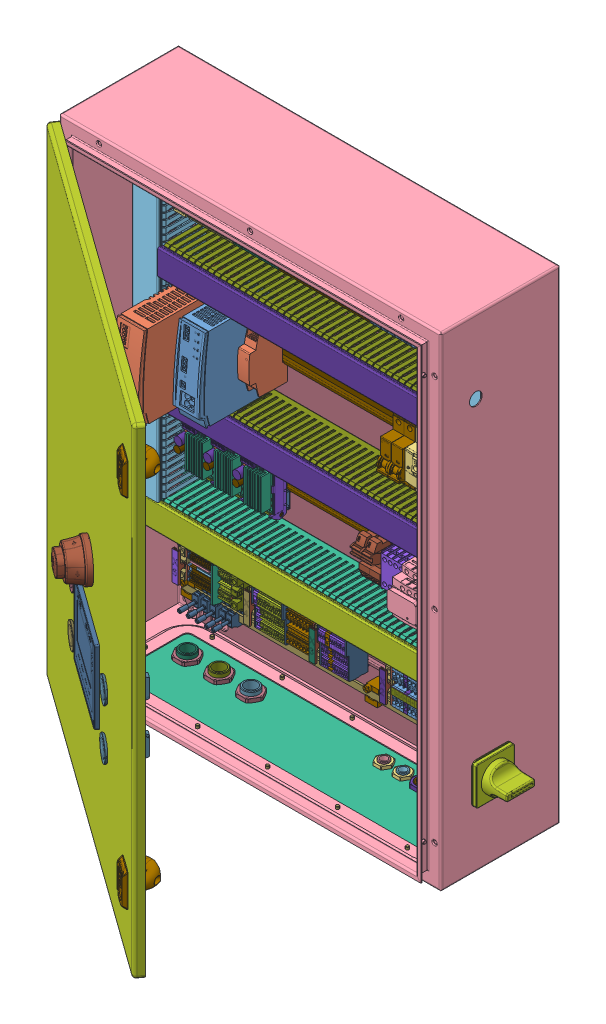
SolidWorks assembly Armoir életrique v46.step, configuration Valor predeterminado. Lengths in mm. (continued)
Components (placement in the parent): (continued)
- EM-241C_v4_1.step-1: EM-241C_v4_1.step [Valor predeterminado] at (-403.6882 -6.6708 82.3602) size (46 89.6 55.6) (continued)
  - DesignRootModel_1.step-1: DesignRootModel_1.step [Valor predeterminado] at origin size (42 72 25.9) (continued)
    - Submodel-CAP0603_47NF_part_0603_5.step-1: Submodel-CAP0603_47NF_part_0603_5.step [Valor predeterminado] at (529.9382 267.464 -26.9602) size (1.75 0.87 0.95) (continued)
      - Submodel-C_UsersTino Hellbergworks3D kokeilujaEM-241Cver4_PCB3DImportedPartModelsCAP 0603.stp_9.step-1: Submodel-C_UsersTino Hellbergworks3D kokeilujaEM-241Cver4_PCB3DImportedPartModelsCAP 0603.stp_9.step [Valor predeterminado] at (96.5835 -11.0791 -43.3309) size (1.75 0.87 0.95) (continued)
        - CAP 0603.stp.step-1: CAP 0603.stp.step [Valor predeterminado] at origin size (1.75 0.87 0.95)
    - Submodel-CAP0603_47NF_part_0603_6.step-1: Submodel-CAP0603_47NF_part_0603_6.step [Valor predeterminado] at (533.9382 268.964 -26.9602) x (0 -1 0) z (0 0 1) size (1.75 0.87 0.95)
      - Submodel-C_UsersTino Hellbergworks3D kokeilujaEM-241Cver4_PCB3DImportedPartModelsCAP 0603.stp_10.step-1: Submodel-C_UsersTino Hellbergworks3D kokeilujaEM-241Cver4_PCB3DImportedPartModelsCAP 0603.stp_10.step [Valor predeterminado] at (96.5835 -11.0791 -43.3309) size (1.75 0.87 0.95)
        - CAP 0603.stp.step-1: CAP 0603.stp.step [Valor predeterminado] at origin size (1.75 0.87 0.95)
    - Submodel-CAP0603_47NF_part_0603_7.step-1: Submodel-CAP0603_47NF_part_0603_7.step [Valor predeterminado] at (536.1882 269.464 -26.9602) x (-1 0 0) z (0 0 1) size (1.75 0.87 0.95)
      - Submodel-C_UsersTino Hellbergworks3D kokeilujaEM-241Cver4_PCB3DImportedPartModelsCAP 0603.stp_11.step-1: Submodel-C_UsersTino Hellbergworks3D kokeilujaEM-241Cver4_PCB3DImportedPartModelsCAP 0603.stp_11.step [Valor predeterminado] at (96.5835 -11.0791 -43.3309) size (1.75 0.87 0.95)
        - CAP 0603.stp.step-1: CAP 0603.stp.step [Valor predeterminado] at origin size (1.75 0.87 0.95)
    - Submodel-LM317LM_SO8_part_SO8_1.step-1: Submodel-LM317LM_SO8_part_SO8_1.step [Valor predeterminado] at (532.4382 283.714 -26.9602) size (4.9 5.78 1.45)
      - Submodel-C_UsersTino Hellbergworks3D kokeilujaEM-241Cver4_PCB3DImportedPartModelsO-8.step_1.step-1: Submodel-C_UsersTino Hellbergworks3D kokeilujaEM-241Cver4_PCB3DImportedPartModelsO-8.step_1.step [Valor predeterminado] at (-1.8923 -2.6289 0) x (0 1 0) z (1 0 0) size (5.78 1.45 4.9)
        - SO-8.step.step-1: SO-8.step.step [Valor predeterminado] at origin size (5.78 1.45 4.9)
    - Submodel-IRLR3705Z_DPAK_NMOS-55V-0.008R-LOGICLEV_part_DPAK_4.step-1: Submodel-IRLR3705Z_DPAK_NMOS-55V-0.008R-LOGICLEV_part_DPAK_4.step [Valor predeterminado] at (547.6882 291.214 -26.9602) x (0 1 0) z (0 0 1) size (6.54 9.94 2.42)
      - Submodel-C_UsersTino Hellbergworks3D kokeilujaEM-241Cver4_PCB3DImportedPartModelsDPAK TO-252.step_4.step-1: Submodel-C_UsersTino Hellbergworks3D kokeilujaEM-241Cver4_PCB3DImportedPartModelsDPAK TO-252.step_4.step [Valor predeterminado] at (0 -1.4833 1.2725) x (1 0 0) z (0 -1 0) size (6.54 2.42 9.94)
        - DPAK TO-252.step.step-1: DPAK TO-252.step.step [Valor predeterminado] at origin size (6.54 2.42 9.94)
    - Submodel-IRLR3705Z_DPAK_NMOS-55V-0.008R-LOGICLEV_part_DPAK_5.step-1: Submodel-IRLR3705Z_DPAK_NMOS-55V-0.008R-LOGICLEV_part_DPAK_5.step [Valor predeterminado] at (533.6882 291.214 -26.9602) x (0 1 0) z (0 0 1) size (6.54 9.94 2.42)
      - Submodel-C_UsersTino Hellbergworks3D kokeilujaEM-241Cver4_PCB3DImportedPartModelsDPAK TO-252.step_5.step-1: Submodel-C_UsersTino Hellbergworks3D kokeilujaEM-241Cver4_PCB3DImportedPartModelsDPAK TO-252.step_5.step [Valor predeterminado] at (0 -1.4833 1.2725) x (1 0 0) z (0 -1 0) size (6.54 2.42 9.94)
        - DPAK TO-252.step.step-1: DPAK TO-252.step.step [Valor predeterminado] at origin size (6.54 2.42 9.94)
    - Submodel-IRLR3705Z_DPAK_NMOS-55V-0.008R-LOGICLEV_part_DPAK_6.step-1: Submodel-IRLR3705Z_DPAK_NMOS-55V-0.008R-LOGICLEV_part_DPAK_6.step [Valor predeterminado] at (547.6882 298.714 -26.9602) x (0 1 0) z (0 0 1) size (6.54 9.94 2.42)
      - Submodel-C_UsersTino Hellbergworks3D kokeilujaEM-241Cver4_PCB3DImportedPartModelsDPAK TO-252.step_6.step-1: Submodel-C_UsersTino Hellbergworks3D kokeilujaEM-241Cver4_PCB3DImportedPartModelsDPAK TO-252.step_6.step [Valor predeterminado] at (0 -1.4833 1.2725) x (1 0 0) z (0 -1 0) size (6.54 2.42 9.94)
        - DPAK TO-252.step.step-1: DPAK TO-252.step.step [Valor predeterminado] at origin size (6.54 2.42 9.94)
    - Submodel-IRLR3705Z_DPAK_NMOS-55V-0.008R-LOGICLEV_part_DPAK_7.step-1: Submodel-IRLR3705Z_DPAK_NMOS-55V-0.008R-LOGICLEV_part_DPAK_7.step [Valor predeterminado] at (533.6882 298.714 -26.9602) x (0 1 0) z (0 0 1) size (6.54 9.94 2.42)
      - Submodel-C_UsersTino Hellbergworks3D kokeilujaEM-241Cver4_PCB3DImportedPartModelsDPAK TO-252.step_7.step-1: Submodel-C_UsersTino Hellbergworks3D kokeilujaEM-241Cver4_PCB3DImportedPartModelsDPAK TO-252.step_7.step [Valor predeterminado] at (0 -1.4833 1.2725) x (1 0 0) z (0 -1 0) size (6.54 2.42 9.94)
        - DPAK TO-252.step.step-1: DPAK TO-252.step.step [Valor predeterminado] at origin size (6.54 2.42 9.94)
    - uid__9223372036854778010.step-1: uid__9223372036854778010.step [Valor predeterminado] at (557.6882 325.214 -28.5602) x (-1 0 0) z (0 0 1) size (42 72 1.6)
  - EM-KP72-42_5_1.step-1: EM-KP72-42_5_1.step [Valor predeterminado] at (537.6882 288.67 -46.3602) x (0 1 0) z (0 0 1) size (89.6 46 37.6)
    - pxc_2907583_00_UM-72-PROFIL-100CM_3D_1.step-1: pxc_2907583_00_UM-72-PROFIL-100CM_3D_1.step [Valor predeterminado] at (0 -67.75 -8.2) x (1 0 0) z (0 -1 0) size (86.8 21.5 40)
      - UM_72-PROFIL_H.Select__00275083.step-1: UM_72-PROFIL_H.Select__00275083.step [Valor predeterminado] at (0 -7.8 -89.5) size (86.8 21.5 40)
    - pxc_2959337_01_UM-72-SE_3D_2.step-1: pxc_2959337_01_UM-72-SE_3D_2.step [Valor predeterminado] at (0 23 -8.5) x (1 0 0) z (0 -1 0) size (89.6 22.8 16)
      - UM_72-SE_H.Select__00276902.step-1: UM_72-SE_H.Select__00276902.step [Valor predeterminado] at (30.8924 14.4135 13) size (89.6 22.8 5)
      - Schr.Lins._3x14-Z_01151118.step-1: Schr.Lins._3x14-Z_01151118.step [Valor predeterminado] at (43.2572 8 73.95) x (1 0 0) z (0 0 -1) size (5.15 5.15 16)
      - Schr.Lins._3x14-Z_01151118.step-2: Schr.Lins._3x14-Z_01151118.step [Valor predeterminado] at (-36.4428 8 73.95) x (1 0 0) z (0 0 -1) size (5.15 5.15 16)
    - pxc_2959337_01_UM-72-SE_3D_3.step-1: pxc_2959337_01_UM-72-SE_3D_3.step [Valor predeterminado] at (0 -23 -8.5) x (-1 0 0) z (0 1 0) size (89.6 22.8 16)
      - UM_72-SE_H.Select__00276902.step-1: UM_72-SE_H.Select__00276902.step [Valor predeterminado] at (30.8924 14.4135 13) size (89.6 22.8 5)
      - Schr.Lins._3x14-Z_01151118.step-1: Schr.Lins._3x14-Z_01151118.step [Valor predeterminado] at (43.2572 8 73.95) x (1 0 0) z (0 0 -1) size (5.15 5.15 16)
      - Schr.Lins._3x14-Z_01151118.step-2: Schr.Lins._3x14-Z_01151118.step [Valor predeterminado] at (-36.4428 8 73.95) x (1 0 0) z (0 0 -1) size (5.15 5.15 16)
    - 39295.step-1: 39295.step [Valor predeterminado] at (0 18 -8.5) x (1 0 0) z (0 -1 0) size (85 18.1 11)
    - 39295.step-2: 39295.step [Valor predeterminado] at (0 -8 -8.5) x (1 0 0) z (0 -1 0) size (85 18.1 11)
- 2903334_RIF_1_RPT_LDP_24DC_2x21-select.step-1: 2903334_RIF_1_RPT_LDP_24DC_2x21-select.step [Valor predeterminado] at (110 -110 -10) x (0 1 0) z (1 0 0) size (104.84 89.77 16.3)
  - 2903334_RIF_1_RPT_LDP_24DC_2x21-select_2.step-1: 2903334_RIF_1_RPT_LDP_24DC_2x21-select_2.step [Valor predeterminado] at (428.6981 37.6678 273.65) x (-0.992546 -0.121869 0) z (0 0 -1) size (95.96 78.66 16.3)
- 3D_G_ST70_XX_03641V.step-1: 3D_G_ST70_XX_03641V.step [Valor predeterminado] at (189.55 608.65 52.3474) size (357.56 90.08 59.8)
  - 3D_G_IK10_XX_91504V.step-1: 3D_G_IK10_XX_91504V.step [Valor predeterminado] at (-299.55 -608.65 -52.3474) size (72.41 90.08 58.26)
    - Body.step-1: Body.step [Valor predeterminado] at (228.0439 619.7488 56.2925) size (72.41 90.08 58.24)
    - Hutschienenadapter.step-1: Hutschienenadapter.step [Valor predeterminado] at (228.0397 633.4963 33.1641) size (14.8 80 4.95)
    - Beschriftung.step-1: Beschriftung.step [Valor predeterminado] at (228.044 619.7489 56.3122) x (1 0 0) z (0 -0.000008 1) size (68.45 86.71 27.67)
  - A5E35094006A_003.step-1: A5E35094006A_003.step [Valor predeterminado] at (0 24.85 -24.85) x (1 0 0) z (0 -1 0) size (71.5 59.7 90)
  - A5E50389032A_001.step-1: A5E50389032A_001.step [Valor predeterminado] at (-0.05 24.85 -24.85) x (1 0 0) z (0 -1 0) size (68.5 29.35 86.02)
  - A5E35212843A_002.step-1: A5E35212843A_002.step [Valor predeterminado] at (18 24.85 -24.85) x (1 0 0) z (0 -1 0) size (0.7 10.8 17.6)
  - 101754.step-1: 101754.step [Valor predeterminado] at (71.5 0.7888 -0.7888) size (79.6 90 58.15)
  - 101754.step-2: 101754.step [Valor predeterminado] at (143 0.7888 -0.7888) size (79.6 90 58.15)
  - 101762.step-1: 101762.step [Valor predeterminado] at (196.5 0.7888 -0.7888) size (43.6 90 58.16)
  - 101762.step-2: 101762.step [Valor predeterminado] at (232 0.7888 -0.7888) size (43.6 90 58.16)
- EM-241C_v4_2.step-1: EM-241C_v4_2.step [Valor predeterminado] at (-329.7091 5.608 81.2521) size (46 89.6 55.6)
  - DesignRootModel_2.step-1: DesignRootModel_2.step [Valor predeterminado] at origin size (42 72 25.9)
    - Submodel-BC846_SOT23_NPN-65V-0.1A_part_simplified_SOT23_4.step-1: Submodel-BC846_SOT23_NPN-65V-0.1A_part_simplified_SOT23_4.step [Valor predeterminado] at (421.2091 273.9352 -25.8521) size (3 2.5 1.1)
      - Submodel-C_UsersTino Hellbergworks3D kokeilujaEM-241Cver4_PCB3DInput_SOT-23.xtd_6.step-1: Submodel-C_UsersTino Hellbergworks3D kokeilujaEM-241Cver4_PCB3DInput_SOT-23.xtd_6.step [Valor predeterminado] at (0 0.1143 0.55) x (-1 0 0) z (0 1 0) size (3 1.1 2.5)
        - SOT-23.step-1: SOT-23.step [Valor predeterminado] at origin size (3 1.1 2.5)
    - Submodel-BC846_SOT23_NPN-65V-0.1A_part_simplified_SOT23_5.step-1: Submodel-BC846_SOT23_NPN-65V-0.1A_part_simplified_SOT23_5.step [Valor predeterminado] at (421.2091 292.4352 -25.8521) x (0 1 0) z (0 0 1) size (3 2.5 1.1)
      - Submodel-C_UsersTino Hellbergworks3D kokeilujaEM-241Cver4_PCB3DInput_SOT-23.xtd_7.step-1: Submodel-C_UsersTino Hellbergworks3D kokeilujaEM-241Cver4_PCB3DInput_SOT-23.xtd_7.step [Valor predeterminado] at (0 0.1143 0.55) x (-1 0 0) z (0 1 0) size (3 1.1 2.5)
        - SOT-23.step-1: SOT-23.step [Valor predeterminado] at origin size (3 1.1 2.5)
    - Submodel-MMUN2211LT1_SOT23_NPN-50V-0.1A-DIGI_part_simplified_SOT23_2.step-1: Submodel-MMUN2211LT1_SOT23_NPN-50V-0.1A-DIGI_part_simplified_SOT23_2.step [Valor predeterminado] at (431.9591 261.1852 -25.8521) size (3 2.5 1.1)
      - Submodel-C_UsersTino Hellbergworks3D kokeilujaEM-241Cver4_PCB3DInput_SOT-23.xtd_8.step-1: Submodel-C_UsersTino Hellbergworks3D kokeilujaEM-241Cver4_PCB3DInput_SOT-23.xtd_8.step [Valor predeterminado] at (0 0.1143 0.55) x (-1 0 0) z (0 1 0) size (3 1.1 2.5)
        - SOT-23.step-1: SOT-23.step [Valor predeterminado] at origin size (3 1.1 2.5)
    - Submodel-RES0805_10R_part_simplified_0805_2.step-1: Submodel-RES0805_10R_part_simplified_0805_2.step [Valor predeterminado] at (400.4591 268.6852 -25.8521) x (0 -1 0) z (0 0 1) size (2 1.25 0.6)
      - Submodel-C_UsersTino Hellbergworks3D kokeilujaEM-241Cver4_PCB3DInput_SRES 0805.xtd_92.step-1: Submodel-C_UsersTino Hellbergworks3D kokeilujaEM-241Cver4_PCB3DInput_SRES 0805.xtd_92.step [Valor predeterminado] at (-0.975 -0.625 0.025) x (1 0 0) z (0 -1 0) size (2 0.6 1.25)
        - RES 0805.step-1: RES 0805.step [Valor predeterminado] at origin size (2 0.6 1.25)
    - Submodel-RES0805_3K9_part_simplified_0805_2.step-1: Submodel-RES0805_3K9_part_simplified_0805_2.step [Valor predeterminado] at (411.7091 264.9352 -25.8521) x (-1 0 0) z (0 0 1) size (2 1.25 0.6)
      - Submodel-C_UsersTino Hellbergworks3D kokeilujaEM-241Cver4_PCB3DInput_SRES 0805.xtd_93.step-1: Submodel-C_UsersTino Hellbergworks3D kokeilujaEM-241Cver4_PCB3DInput_SRES 0805.xtd_93.step [Valor predeterminado] at (-0.975 -0.625 0.025) x (1 0 0) z (0 -1 0) size (2 0.6 1.25)
        - RES 0805.step-1: RES 0805.step [Valor predeterminado] at origin size (2 0.6 1.25)
    - Submodel-RES0805_22K_part_simplified_0805_4.step-1: Submodel-RES0805_22K_part_simplified_0805_4.step [Valor predeterminado] at (419.9591 252.4352 -25.8521) x (0 1 0) z (0 0 1) size (2 1.25 0.6)
      - Submodel-C_UsersTino Hellbergworks3D kokeilujaEM-241Cver4_PCB3DInput_SRES 0805.xtd_94.step-1: Submodel-C_UsersTino Hellbergworks3D kokeilujaEM-241Cver4_PCB3DInput_SRES 0805.xtd_94.step [Valor predeterminado] at (-0.975 -0.625 0.025) x (1 0 0) z (0 -1 0) size (2 0.6 1.25)
        - RES 0805.step-1: RES 0805.step [Valor predeterminado] at origin size (2 0.6 1.25)
    - Submodel-RES0805_22K_part_simplified_0805_5.step-1: Submodel-RES0805_22K_part_simplified_0805_5.step [Valor predeterminado] at (411.7091 263.1852 -25.8521) x (-1 0 0) z (0 0 1) size (2 1.25 0.6)
      - Submodel-C_UsersTino Hellbergworks3D kokeilujaEM-241Cver4_PCB3DInput_SRES 0805.xtd_95.step-1: Submodel-C_UsersTino Hellbergworks3D kokeilujaEM-241Cver4_PCB3DInput_SRES 0805.xtd_95.step [Valor predeterminado] at (-0.975 -0.625 0.025) x (1 0 0) z (0 -1 0) size (2 0.6 1.25)
        - RES 0805.step-1: RES 0805.step [Valor predeterminado] at origin size (2 0.6 1.25)
    - Submodel-RES0805_1K2_part_simplified_0805_4.step-1: Submodel-RES0805_1K2_part_simplified_0805_4.step [Valor predeterminado] at (411.7091 266.6852 -25.8521) x (-1 0 0) z (0 0 1) size (2 1.25 0.6)
      - Submodel-C_UsersTino Hellbergworks3D kokeilujaEM-241Cver4_PCB3DInput_SRES 0805.xtd_96.step-1: Submodel-C_UsersTino Hellbergworks3D kokeilujaEM-241Cver4_PCB3DInput_SRES 0805.xtd_96.step [Valor predeterminado] at (-0.975 -0.625 0.025) x (1 0 0) z (0 -1 0) size (2 0.6 1.25)
        - RES 0805.step-1: RES 0805.step [Valor predeterminado] at origin size (2 0.6 1.25)
    - Submodel-RES0805_1K2_part_simplified_0805_5.step-1: Submodel-RES0805_1K2_part_simplified_0805_5.step [Valor predeterminado] at (412.2091 293.1852 -25.8521) x (-1 0 0) z (0 0 1) size (2 1.25 0.6)
      - Submodel-C_UsersTino Hellbergworks3D kokeilujaEM-241Cver4_PCB3DInput_SRES 0805.xtd_97.step-1: Submodel-C_UsersTino Hellbergworks3D kokeilujaEM-241Cver4_PCB3DInput_SRES 0805.xtd_97.step [Valor predeterminado] at (-0.975 -0.625 0.025) x (1 0 0) z (0 -1 0) size (2 0.6 1.25)
        - RES 0805.step-1: RES 0805.step [Valor predeterminado] at origin size (2 0.6 1.25)
    - Submodel-RES0805_47K_part_simplified_0805_28.step-1: Submodel-RES0805_47K_part_simplified_0805_28.step [Valor predeterminado] at (434.4591 267.1852 -25.8521) x (-1 0 0) z (0 0 1) size (2 1.25 0.6)
      - Submodel-C_UsersTino Hellbergworks3D kokeilujaEM-241Cver4_PCB3DInput_SRES 0805.xtd_98.step-1: Submodel-C_UsersTino Hellbergworks3D kokeilujaEM-241Cver4_PCB3DInput_SRES 0805.xtd_98.step [Valor predeterminado] at (-0.975 -0.625 0.025) x (1 0 0) z (0 -1 0) size (2 0.6 1.25)
        - RES 0805.step-1: RES 0805.step [Valor predeterminado] at origin size (2 0.6 1.25)
    - Submodel-RES0805_47K_part_simplified_0805_29.step-1: Submodel-RES0805_47K_part_simplified_0805_29.step [Valor predeterminado] at (404.7091 257.1852 -25.8521) size (2 1.25 0.6)
      - Submodel-C_UsersTino Hellbergworks3D kokeilujaEM-241Cver4_PCB3DInput_SRES 0805.xtd_99.step-1: Submodel-C_UsersTino Hellbergworks3D kokeilujaEM-241Cver4_PCB3DInput_SRES 0805.xtd_99.step [Valor predeterminado] at (-0.975 -0.625 0.025) x (1 0 0) z (0 -1 0) size (2 0.6 1.25)
        - RES 0805.step-1: RES 0805.step [Valor predeterminado] at origin size (2 0.6 1.25)
    - Submodel-RES0805_47K_part_simplified_0805_30.step-1: Submodel-RES0805_47K_part_simplified_0805_30.step [Valor predeterminado] at (404.2091 253.4352 -25.8521) x (-1 0 0) z (0 0 1) size (2 1.25 0.6)
      - Submodel-C_UsersTino Hellbergworks3D kokeilujaEM-241Cver4_PCB3DInput_SRES 0805.xtd_100.step-1: Submodel-C_UsersTino Hellbergworks3D kokeilujaEM-241Cver4_PCB3DInput_SRES 0805.xtd_100.step [Valor predeterminado] at (-0.975 -0.625 0.025) x (1 0 0) z (0 -1 0) size (2 0.6 1.25)
        - RES 0805.step-1: RES 0805.step [Valor predeterminado] at origin size (2 0.6 1.25)
    - Submodel-RES0805_47K_part_simplified_0805_31.step-1: Submodel-RES0805_47K_part_simplified_0805_31.step [Valor predeterminado] at (404.2091 251.4352 -25.8521) x (-1 0 0) z (0 0 1) size (2 1.25 0.6)
      - Submodel-C_UsersTino Hellbergworks3D kokeilujaEM-241Cver4_PCB3DInput_SRES 0805.xtd_101.step-1: Submodel-C_UsersTino Hellbergworks3D kokeilujaEM-241Cver4_PCB3DInput_SRES 0805.xtd_101.step [Valor predeterminado] at (-0.975 -0.625 0.025) x (1 0 0) z (0 -1 0) size (2 0.6 1.25)
        - RES 0805.step-1: RES 0805.step [Valor predeterminado] at origin size (2 0.6 1.25)
    - Submodel-RES0805_47K_part_simplified_0805_32.step-1: Submodel-RES0805_47K_part_simplified_0805_32.step [Valor predeterminado] at (408.2091 257.1852 -25.8521) size (2 1.25 0.6)
      - Submodel-C_UsersTino Hellbergworks3D kokeilujaEM-241Cver4_PCB3DInput_SRES 0805.xtd_102.step-1: Submodel-C_UsersTino Hellbergworks3D kokeilujaEM-241Cver4_PCB3DInput_SRES 0805.xtd_102.step [Valor predeterminado] at (-0.975 -0.625 0.025) x (1 0 0) z (0 -1 0) size (2 0.6 1.25)
        - RES 0805.step-1: RES 0805.step [Valor predeterminado] at origin size (2 0.6 1.25)
    - Submodel-RES0805_47K_part_simplified_0805_33.step-1: Submodel-RES0805_47K_part_simplified_0805_33.step [Valor predeterminado] at (407.9591 253.4352 -25.8521) x (-1 0 0) z (0 0 1) size (2 1.25 0.6)
      - Submodel-C_UsersTino Hellbergworks3D kokeilujaEM-241Cver4_PCB3DInput_SRES 0805.xtd_103.step-1: Submodel-C_UsersTino Hellbergworks3D kokeilujaEM-241Cver4_PCB3DInput_SRES 0805.xtd_103.step [Valor predeterminado] at (-0.975 -0.625 0.025) x (1 0 0) z (0 -1 0) size (2 0.6 1.25)
        - RES 0805.step-1: RES 0805.step [Valor predeterminado] at origin size (2 0.6 1.25)
    - Submodel-RES0805_47K_part_simplified_0805_34.step-1: Submodel-RES0805_47K_part_simplified_0805_34.step [Valor predeterminado] at (407.9591 251.4352 -25.8521) x (-1 0 0) z (0 0 1) size (2 1.25 0.6)
      - Submodel-C_UsersTino Hellbergworks3D kokeilujaEM-241Cver4_PCB3DInput_SRES 0805.xtd_104.step-1: Submodel-C_UsersTino Hellbergworks3D kokeilujaEM-241Cver4_PCB3DInput_SRES 0805.xtd_104.step [Valor predeterminado] at (-0.975 -0.625 0.025) x (1 0 0) z (0 -1 0) size (2 0.6 1.25)
        - RES 0805.step-1: RES 0805.step [Valor predeterminado] at origin size (2 0.6 1.25)
    - Submodel-RES0805_47K_part_simplified_0805_35.step-1: Submodel-RES0805_47K_part_simplified_0805_35.step [Valor predeterminado] at (412.4591 256.4352 -25.8521) x (0 1 0) z (0 0 1) size (2 1.25 0.6)
      - Submodel-C_UsersTino Hellbergworks3D kokeilujaEM-241Cver4_PCB3DInput_SRES 0805.xtd_105.step-1: Submodel-C_UsersTino Hellbergworks3D kokeilujaEM-241Cver4_PCB3DInput_SRES 0805.xtd_105.step [Valor predeterminado] at (-0.975 -0.625 0.025) x (1 0 0) z (0 -1 0) size (2 0.6 1.25)
        - RES 0805.step-1: RES 0805.step [Valor predeterminado] at origin size (2 0.6 1.25)
    - Submodel-RES0805_47K_part_simplified_0805_36.step-1: Submodel-RES0805_47K_part_simplified_0805_36.step [Valor predeterminado] at (411.7091 253.4352 -25.8521) x (-1 0 0) z (0 0 1) size (2 1.25 0.6)
      - Submodel-C_UsersTino Hellbergworks3D kokeilujaEM-241Cver4_PCB3DInput_SRES 0805.xtd_106.step-1: Submodel-C_UsersTino Hellbergworks3D kokeilujaEM-241Cver4_PCB3DInput_SRES 0805.xtd_106.step [Valor predeterminado] at (-0.975 -0.625 0.025) x (1 0 0) z (0 -1 0) size (2 0.6 1.25)
        - RES 0805.step-1: RES 0805.step [Valor predeterminado] at origin size (2 0.6 1.25)
    - Submodel-RES0805_47K_part_simplified_0805_37.step-1: Submodel-RES0805_47K_part_simplified_0805_37.step [Valor predeterminado] at (411.7091 251.4352 -25.8521) x (-1 0 0) z (0 0 1) size (2 1.25 0.6)
      - Submodel-C_UsersTino Hellbergworks3D kokeilujaEM-241Cver4_PCB3DInput_SRES 0805.xtd_107.step-1: Submodel-C_UsersTino Hellbergworks3D kokeilujaEM-241Cver4_PCB3DInput_SRES 0805.xtd_107.step [Valor predeterminado] at (-0.975 -0.625 0.025) x (1 0 0) z (0 -1 0) size (2 0.6 1.25)
        - RES 0805.step-1: RES 0805.step [Valor predeterminado] at origin size (2 0.6 1.25)
    - Submodel-RES0805_47K_part_simplified_0805_38.step-1: Submodel-RES0805_47K_part_simplified_0805_38.step [Valor predeterminado] at (417.7091 255.6852 -25.8521) size (2 1.25 0.6)
      - Submodel-C_UsersTino Hellbergworks3D kokeilujaEM-241Cver4_PCB3DInput_SRES 0805.xtd_108.step-1: Submodel-C_UsersTino Hellbergworks3D kokeilujaEM-241Cver4_PCB3DInput_SRES 0805.xtd_108.step [Valor predeterminado] at (-0.975 -0.625 0.025) x (1 0 0) z (0 -1 0) size (2 0.6 1.25)
        - RES 0805.step-1: RES 0805.step [Valor predeterminado] at origin size (2 0.6 1.25)
    - Submodel-RES0805_47K_part_simplified_0805_39.step-1: Submodel-RES0805_47K_part_simplified_0805_39.step [Valor predeterminado] at (415.4591 253.4352 -25.8521) size (2 1.25 0.6)
      - Submodel-C_UsersTino Hellbergworks3D kokeilujaEM-241Cver4_PCB3DInput_SRES 0805.xtd_109.step-1: Submodel-C_UsersTino Hellbergworks3D kokeilujaEM-241Cver4_PCB3DInput_SRES 0805.xtd_109.step [Valor predeterminado] at (-0.975 -0.625 0.025) x (1 0 0) z (0 -1 0) size (2 0.6 1.25)
        - RES 0805.step-1: RES 0805.step [Valor predeterminado] at origin size (2 0.6 1.25)
    - Submodel-RES0805_47K_part_simplified_0805_40.step-1: Submodel-RES0805_47K_part_simplified_0805_40.step [Valor predeterminado] at (415.4591 251.4352 -25.8521) size (2 1.25 0.6)
      - Submodel-C_UsersTino Hellbergworks3D kokeilujaEM-241Cver4_PCB3DInput_SRES 0805.xtd_110.step-1: Submodel-C_UsersTino Hellbergworks3D kokeilujaEM-241Cver4_PCB3DInput_SRES 0805.xtd_110.step [Valor predeterminado] at (-0.975 -0.625 0.025) x (1 0 0) z (0 -1 0) size (2 0.6 1.25)
        - RES 0805.step-1: RES 0805.step [Valor predeterminado] at origin size (2 0.6 1.25)
    - Submodel-RES0805_47K_part_simplified_0805_41.step-1: Submodel-RES0805_47K_part_simplified_0805_41.step [Valor predeterminado] at (435.4591 258.6852 -25.8521) x (-1 0 0) z (0 0 1) size (2 1.25 0.6)
      - Submodel-C_UsersTino Hellbergworks3D kokeilujaEM-241Cver4_PCB3DInput_SRES 0805.xtd_111.step-1: Submodel-C_UsersTino Hellbergworks3D kokeilujaEM-241Cver4_PCB3DInput_SRES 0805.xtd_111.step [Valor predeterminado] at (-0.975 -0.625 0.025) x (1 0 0) z (0 -1 0) size (2 0.6 1.25)
        - RES 0805.step-1: RES 0805.step [Valor predeterminado] at origin size (2 0.6 1.25)
    - Submodel-RES0805_1M_part_simplified_0805_2.step-1: Submodel-RES0805_1M_part_simplified_0805_2.step [Valor predeterminado] at (419.4591 269.6852 -25.8521) x (0 -1 0) z (0 0 1) size (2 1.25 0.6)
      - Submodel-C_UsersTino Hellbergworks3D kokeilujaEM-241Cver4_PCB3DInput_SRES 0805.xtd_112.step-1: Submodel-C_UsersTino Hellbergworks3D kokeilujaEM-241Cver4_PCB3DInput_SRES 0805.xtd_112.step [Valor predeterminado] at (-0.975 -0.625 0.025) x (1 0 0) z (0 -1 0) size (2 0.6 1.25)
        - RES 0805.step-1: RES 0805.step [Valor predeterminado] at origin size (2 0.6 1.25)
    - Submodel-RES0805_22R_part_simplified_0805_4.step-1: Submodel-RES0805_22R_part_simplified_0805_4.step [Valor predeterminado] at (415.9591 293.1852 -25.8521) x (-1 0 0) z (0 0 1) size (2 1.25 0.6)
      - Submodel-C_UsersTino Hellbergworks3D kokeilujaEM-241Cver4_PCB3DInput_SRES 0805.xtd_113.step-1: Submodel-C_UsersTino Hellbergworks3D kokeilujaEM-241Cver4_PCB3DInput_SRES 0805.xtd_113.step [Valor predeterminado] at (-0.975 -0.625 0.025) x (1 0 0) z (0 -1 0) size (2 0.6 1.25)
        - RES 0805.step-1: RES 0805.step [Valor predeterminado] at origin size (2 0.6 1.25)
    - Submodel-RES0805_22R_part_simplified_0805_5.step-1: Submodel-RES0805_22R_part_simplified_0805_5.step [Valor predeterminado] at (421.4591 269.6852 -25.8521) x (0 -1 0) z (0 0 1) size (2 1.25 0.6)
      - Submodel-C_UsersTino Hellbergworks3D kokeilujaEM-241Cver4_PCB3DInput_SRES 0805.xtd_114.step-1: Submodel-C_UsersTino Hellbergworks3D kokeilujaEM-241Cver4_PCB3DInput_SRES 0805.xtd_114.step [Valor predeterminado] at (-0.975 -0.625 0.025) x (1 0 0) z (0 -1 0) size (2 0.6 1.25)
        - RES 0805.step-1: RES 0805.step [Valor predeterminado] at origin size (2 0.6 1.25)
    - Submodel-RES0805_100K_part_simplified_0805_14.step-1: Submodel-RES0805_100K_part_simplified_0805_14.step [Valor predeterminado] at (431.9591 258.6852 -25.8521) x (-1 0 0) z (0 0 1) size (2 1.25 0.6)
      - Submodel-C_UsersTino Hellbergworks3D kokeilujaEM-241Cver4_PCB3DInput_SRES 0805.xtd_115.step-1: Submodel-C_UsersTino Hellbergworks3D kokeilujaEM-241Cver4_PCB3DInput_SRES 0805.xtd_115.step [Valor predeterminado] at (-0.975 -0.625 0.025) x (1 0 0) z (0 -1 0) size (2 0.6 1.25)
        - RES 0805.step-1: RES 0805.step [Valor predeterminado] at origin size (2 0.6 1.25)
    - Submodel-RES0805_100K_part_simplified_0805_15.step-1: Submodel-RES0805_100K_part_simplified_0805_15.step [Valor predeterminado] at (418.7091 273.6852 -25.8521) x (0 1 0) z (0 0 1) size (2 1.25 0.6)
      - Submodel-C_UsersTino Hellbergworks3D kokeilujaEM-241Cver4_PCB3DInput_SRES 0805.xtd_116.step-1: Submodel-C_UsersTino Hellbergworks3D kokeilujaEM-241Cver4_PCB3DInput_SRES 0805.xtd_116.step [Valor predeterminado] at (-0.975 -0.625 0.025) x (1 0 0) z (0 -1 0) size (2 0.6 1.25)
        - RES 0805.step-1: RES 0805.step [Valor predeterminado] at origin size (2 0.6 1.25)
    - Submodel-RES0805_100K_part_simplified_0805_16.step-1: Submodel-RES0805_100K_part_simplified_0805_16.step [Valor predeterminado] at (415.9591 290.9352 -25.8521) size (2 1.25 0.6)
      - Submodel-C_UsersTino Hellbergworks3D kokeilujaEM-241Cver4_PCB3DInput_SRES 0805.xtd_117.step-1: Submodel-C_UsersTino Hellbergworks3D kokeilujaEM-241Cver4_PCB3DInput_SRES 0805.xtd_117.step [Valor predeterminado] at (-0.975 -0.625 0.025) x (1 0 0) z (0 -1 0) size (2 0.6 1.25)
        - RES 0805.step-1: RES 0805.step [Valor predeterminado] at origin size (2 0.6 1.25)
    - Submodel-RES0805_100K_part_simplified_0805_17.step-1: Submodel-RES0805_100K_part_simplified_0805_17.step [Valor predeterminado] at (398.7091 268.6852 -25.8521) x (0 -1 0) z (0 0 1) size (2 1.25 0.6)
      - Submodel-C_UsersTino Hellbergworks3D kokeilujaEM-241Cver4_PCB3DInput_SRES 0805.xtd_118.step-1: Submodel-C_UsersTino Hellbergworks3D kokeilujaEM-241Cver4_PCB3DInput_SRES 0805.xtd_118.step [Valor predeterminado] at (-0.975 -0.625 0.025) x (1 0 0) z (0 -1 0) size (2 0.6 1.25)
        - RES 0805.step-1: RES 0805.step [Valor predeterminado] at origin size (2 0.6 1.25)
    - Submodel-RES0805_100K_part_simplified_0805_18.step-1: Submodel-RES0805_100K_part_simplified_0805_18.step [Valor predeterminado] at (405.9591 262.9352 -25.8521) x (0 1 0) z (0 0 1) size (2 1.25 0.6)
      - Submodel-C_UsersTino Hellbergworks3D kokeilujaEM-241Cver4_PCB3DInput_SRES 0805.xtd_119.step-1: Submodel-C_UsersTino Hellbergworks3D kokeilujaEM-241Cver4_PCB3DInput_SRES 0805.xtd_119.step [Valor predeterminado] at (-0.975 -0.625 0.025) x (1 0 0) z (0 -1 0) size (2 0.6 1.25)
        - RES 0805.step-1: RES 0805.step [Valor predeterminado] at origin size (2 0.6 1.25)
    - Submodel-RES0805_100K_part_simplified_0805_19.step-1: Submodel-RES0805_100K_part_simplified_0805_19.step [Valor predeterminado] at (431.4591 251.9352 -25.8521) x (0 -1 0) z (0 0 1) size (2 1.25 0.6)
      - Submodel-C_UsersTino Hellbergworks3D kokeilujaEM-241Cver4_PCB3DInput_SRES 0805.xtd_120.step-1: Submodel-C_UsersTino Hellbergworks3D kokeilujaEM-241Cver4_PCB3DInput_SRES 0805.xtd_120.step [Valor predeterminado] at (-0.975 -0.625 0.025) x (1 0 0) z (0 -1 0) size (2 0.6 1.25)
        - RES 0805.step-1: RES 0805.step [Valor predeterminado] at origin size (2 0.6 1.25)
    - Submodel-RES0805_100K_part_simplified_0805_20.step-1: Submodel-RES0805_100K_part_simplified_0805_20.step [Valor predeterminado] at (418.2091 252.4352 -25.8521) x (0 1 0) z (0 0 1) size (2 1.25 0.6)
      - Submodel-C_UsersTino Hellbergworks3D kokeilujaEM-241Cver4_PCB3DInput_SRES 0805.xtd_121.step-1: Submodel-C_UsersTino Hellbergworks3D kokeilujaEM-241Cver4_PCB3DInput_SRES 0805.xtd_121.step [Valor predeterminado] at (-0.975 -0.625 0.025) x (1 0 0) z (0 -1 0) size (2 0.6 1.25)
        - RES 0805.step-1: RES 0805.step [Valor predeterminado] at origin size (2 0.6 1.25)
    - Submodel-RES0805_10K_part_simplified_0805_8.step-1: Submodel-RES0805_10K_part_simplified_0805_8.step [Valor predeterminado] at (435.4591 252.9352 -25.8521) x (-1 0 0) z (0 0 1) size (2 1.25 0.6)
      - Submodel-C_UsersTino Hellbergworks3D kokeilujaEM-241Cver4_PCB3DInput_SRES 0805.xtd_122.step-1: Submodel-C_UsersTino Hellbergworks3D kokeilujaEM-241Cver4_PCB3DInput_SRES 0805.xtd_122.step [Valor predeterminado] at (-0.975 -0.625 0.025) x (1 0 0) z (0 -1 0) size (2 0.6 1.25)
        - RES 0805.step-1: RES 0805.step [Valor predeterminado] at origin size (2 0.6 1.25)
    - Submodel-RES0805_10K_part_simplified_0805_9.step-1: Submodel-RES0805_10K_part_simplified_0805_9.step [Valor predeterminado] at (435.4591 262.1852 -25.8521) size (2 1.25 0.6)
      - Submodel-C_UsersTino Hellbergworks3D kokeilujaEM-241Cver4_PCB3DInput_SRES 0805.xtd_123.step-1: Submodel-C_UsersTino Hellbergworks3D kokeilujaEM-241Cver4_PCB3DInput_SRES 0805.xtd_123.step [Valor predeterminado] at (-0.975 -0.625 0.025) x (1 0 0) z (0 -1 0) size (2 0.6 1.25)
        - RES 0805.step-1: RES 0805.step [Valor predeterminado] at origin size (2 0.6 1.25)
    - Submodel-RES0805_10K_part_simplified_0805_10.step-1: Submodel-RES0805_10K_part_simplified_0805_10.step [Valor predeterminado] at (435.4591 260.4352 -25.8521) size (2 1.25 0.6)
      - Submodel-C_UsersTino Hellbergworks3D kokeilujaEM-241Cver4_PCB3DInput_SRES 0805.xtd_124.step-1: Submodel-C_UsersTino Hellbergworks3D kokeilujaEM-241Cver4_PCB3DInput_SRES 0805.xtd_124.step [Valor predeterminado] at (-0.975 -0.625 0.025) x (1 0 0) z (0 -1 0) size (2 0.6 1.25)
        - RES 0805.step-1: RES 0805.step [Valor predeterminado] at origin size (2 0.6 1.25)
    - Submodel-RES0805_10K_part_simplified_0805_11.step-1: Submodel-RES0805_10K_part_simplified_0805_11.step [Valor predeterminado] at (424.7091 252.4352 -25.8521) x (0 1 0) z (0 0 1) size (2 1.25 0.6)
      - Submodel-C_UsersTino Hellbergworks3D kokeilujaEM-241Cver4_PCB3DInput_SRES 0805.xtd_125.step-1: Submodel-C_UsersTino Hellbergworks3D kokeilujaEM-241Cver4_PCB3DInput_SRES 0805.xtd_125.step [Valor predeterminado] at (-0.975 -0.625 0.025) x (1 0 0) z (0 -1 0) size (2 0.6 1.25)
        - RES 0805.step-1: RES 0805.step [Valor predeterminado] at origin size (2 0.6 1.25)
    - Submodel-RES1206_10R_part_simplified_1206_2.step-1: Submodel-RES1206_10R_part_simplified_1206_2.step [Valor predeterminado] at (428.9591 248.6852 -25.8521) size (3.35 1.73 0.85)
      - Submodel-C_UsersTino Hellbergworks3D kokeilujaEM-241Cver4_PCB3DInput_SRES-1206.xtd_4.step-1: Submodel-C_UsersTino Hellbergworks3D kokeilujaEM-241Cver4_PCB3DInput_SRES-1206.xtd_4.step [Valor predeterminado] x (1 0 0) z (0 -1 0) size (3.35 0.85 1.73)
        - RES-1206.step-1: RES-1206.step [Valor predeterminado] at origin size (3.35 0.85 1.73)
    - Submodel-RES0805_1K_part_simplified_0805_4.step-1: Submodel-RES0805_1K_part_simplified_0805_4.step [Valor predeterminado] at (435.4591 251.1852 -25.8521) x (-1 0 0) z (0 0 1) size (2 1.25 0.6)
      - Submodel-C_UsersTino Hellbergworks3D kokeilujaEM-241Cver4_PCB3DInput_SRES 0805.xtd_126.step-1: Submodel-C_UsersTino Hellbergworks3D kokeilujaEM-241Cver4_PCB3DInput_SRES 0805.xtd_126.step [Valor predeterminado] at (-0.975 -0.625 0.025) x (1 0 0) z (0 -1 0) size (2 0.6 1.25)
        - RES 0805.step-1: RES 0805.step [Valor predeterminado] at origin size (2 0.6 1.25)
    - Submodel-RES0805_1K_part_simplified_0805_5.step-1: Submodel-RES0805_1K_part_simplified_0805_5.step [Valor predeterminado] at (428.9591 273.4352 -25.8521) x (0 1 0) z (0 0 1) size (2 1.25 0.6)
      - Submodel-C_UsersTino Hellbergworks3D kokeilujaEM-241Cver4_PCB3DInput_SRES 0805.xtd_127.step-1: Submodel-C_UsersTino Hellbergworks3D kokeilujaEM-241Cver4_PCB3DInput_SRES 0805.xtd_127.step [Valor predeterminado] at (-0.975 -0.625 0.025) x (1 0 0) z (0 -1 0) size (2 0.6 1.25)
        - RES 0805.step-1: RES 0805.step [Valor predeterminado] at origin size (2 0.6 1.25)
    - Submodel-RES1206_100R_part_simplified_1206_2.step-1: Submodel-RES1206_100R_part_simplified_1206_2.step [Valor predeterminado] at (428.2091 252.4352 -25.8521) x (0 1 0) z (0 0 1) size (3.35 1.73 0.85)
      - Submodel-C_UsersTino Hellbergworks3D kokeilujaEM-241Cver4_PCB3DInput_SRES-1206.xtd_5.step-1: Submodel-C_UsersTino Hellbergworks3D kokeilujaEM-241Cver4_PCB3DInput_SRES-1206.xtd_5.step [Valor predeterminado] x (1 0 0) z (0 -1 0) size (3.35 0.85 1.73)
        - RES-1206.step-1: RES-1206.step [Valor predeterminado] at origin size (3.35 0.85 1.73)
    - Submodel-RES0805_220R_part_simplified_0805_4.step-1: Submodel-RES0805_220R_part_simplified_0805_4.step [Valor predeterminado] at (435.4591 273.9352 -25.8521) x (0 1 0) z (0 0 1) size (2 1.25 0.6)
      - Submodel-C_UsersTino Hellbergworks3D kokeilujaEM-241Cver4_PCB3DInput_SRES 0805.xtd_128.step-1: Submodel-C_UsersTino Hellbergworks3D kokeilujaEM-241Cver4_PCB3DInput_SRES 0805.xtd_128.step [Valor predeterminado] at (-0.975 -0.625 0.025) x (1 0 0) z (0 -1 0) size (2 0.6 1.25)
        - RES 0805.step-1: RES 0805.step [Valor predeterminado] at origin size (2 0.6 1.25)
    - Submodel-RES0805_220R_part_simplified_0805_5.step-1: Submodel-RES0805_220R_part_simplified_0805_5.step [Valor predeterminado] at (433.4591 273.9352 -25.8521) x (0 1 0) z (0 0 1) size (2 1.25 0.6)
      - Submodel-C_UsersTino Hellbergworks3D kokeilujaEM-241Cver4_PCB3DInput_SRES 0805.xtd_129.step-1: Submodel-C_UsersTino Hellbergworks3D kokeilujaEM-241Cver4_PCB3DInput_SRES 0805.xtd_129.step [Valor predeterminado] at (-0.975 -0.625 0.025) x (1 0 0) z (0 -1 0) size (2 0.6 1.25)
        - RES 0805.step-1: RES 0805.step [Valor predeterminado] at origin size (2 0.6 1.25)
    - Submodel-RES0805_2K2_part_simplified_0805_14.step-1: Submodel-RES0805_2K2_part_simplified_0805_14.step [Valor predeterminado] at (396.9591 268.6852 -25.8521) x (0 -1 0) z (0 0 1) size (2 1.25 0.6)
      - Submodel-C_UsersTino Hellbergworks3D kokeilujaEM-241Cver4_PCB3DInput_SRES 0805.xtd_130.step-1: Submodel-C_UsersTino Hellbergworks3D kokeilujaEM-241Cver4_PCB3DInput_SRES 0805.xtd_130.step [Valor predeterminado] at (-0.975 -0.625 0.025) x (1 0 0) z (0 -1 0) size (2 0.6 1.25)
        - RES 0805.step-1: RES 0805.step [Valor predeterminado] at origin size (2 0.6 1.25)
    - Submodel-RES0805_2K2_part_simplified_0805_15.step-1: Submodel-RES0805_2K2_part_simplified_0805_15.step [Valor predeterminado] at (422.9591 252.4352 -25.8521) x (0 -1 0) z (0 0 1) size (2 1.25 0.6)
      - Submodel-C_UsersTino Hellbergworks3D kokeilujaEM-241Cver4_PCB3DInput_SRES 0805.xtd_131.step-1: Submodel-C_UsersTino Hellbergworks3D kokeilujaEM-241Cver4_PCB3DInput_SRES 0805.xtd_131.step [Valor predeterminado] at (-0.975 -0.625 0.025) x (1 0 0) z (0 -1 0) size (2 0.6 1.25)
        - RES 0805.step-1: RES 0805.step [Valor predeterminado] at origin size (2 0.6 1.25)
    - Submodel-RES0805_2K2_part_simplified_0805_16.step-1: Submodel-RES0805_2K2_part_simplified_0805_16.step [Valor predeterminado] at (399.2091 248.9352 -25.8521) x (-1 0 0) z (0 0 1) size (2 1.25 0.6)
      - Submodel-C_UsersTino Hellbergworks3D kokeilujaEM-241Cver4_PCB3DInput_SRES 0805.xtd_132.step-1: Submodel-C_UsersTino Hellbergworks3D kokeilujaEM-241Cver4_PCB3DInput_SRES 0805.xtd_132.step [Valor predeterminado] at (-0.975 -0.625 0.025) x (1 0 0) z (0 -1 0) size (2 0.6 1.25)
        - RES 0805.step-1: RES 0805.step [Valor predeterminado] at origin size (2 0.6 1.25)
    - Submodel-RES0805_2K2_part_simplified_0805_17.step-1: Submodel-RES0805_2K2_part_simplified_0805_17.step [Valor predeterminado] at (404.7091 259.4352 -25.8521) x (-1 0 0) z (0 0 1) size (2 1.25 0.6)
      - Submodel-C_UsersTino Hellbergworks3D kokeilujaEM-241Cver4_PCB3DInput_SRES 0805.xtd_133.step-1: Submodel-C_UsersTino Hellbergworks3D kokeilujaEM-241Cver4_PCB3DInput_SRES 0805.xtd_133.step [Valor predeterminado] at (-0.975 -0.625 0.025) x (1 0 0) z (0 -1 0) size (2 0.6 1.25)
        - RES 0805.step-1: RES 0805.step [Valor predeterminado] at origin size (2 0.6 1.25)
    - Submodel-RES0805_2K2_part_simplified_0805_18.step-1: Submodel-RES0805_2K2_part_simplified_0805_18.step [Valor predeterminado] at (430.9591 273.4352 -25.8521) x (0 1 0) z (0 0 1) size (2 1.25 0.6)
      - Submodel-C_UsersTino Hellbergworks3D kokeilujaEM-241Cver4_PCB3DInput_SRES 0805.xtd_134.step-1: Submodel-C_UsersTino Hellbergworks3D kokeilujaEM-241Cver4_PCB3DInput_SRES 0805.xtd_134.step [Valor predeterminado] at (-0.975 -0.625 0.025) x (1 0 0) z (0 -1 0) size (2 0.6 1.25)
        - RES 0805.step-1: RES 0805.step [Valor predeterminado] at origin size (2 0.6 1.25)
    - Submodel-RES0805_2K2_part_simplified_0805_19.step-1: Submodel-RES0805_2K2_part_simplified_0805_19.step [Valor predeterminado] at (433.9591 271.4352 -25.8521) x (-1 0 0) z (0 0 1) size (2 1.25 0.6)
      - Submodel-C_UsersTino Hellbergworks3D kokeilujaEM-241Cver4_PCB3DInput_SRES 0805.xtd_135.step-1: Submodel-C_UsersTino Hellbergworks3D kokeilujaEM-241Cver4_PCB3DInput_SRES 0805.xtd_135.step [Valor predeterminado] at (-0.975 -0.625 0.025) x (1 0 0) z (0 -1 0) size (2 0.6 1.25)
        - RES 0805.step-1: RES 0805.step [Valor predeterminado] at origin size (2 0.6 1.25)
    - Submodel-RES0805_2K2_part_simplified_0805_20.step-1: Submodel-RES0805_2K2_part_simplified_0805_20.step [Valor predeterminado] at (430.4591 245.9352 -25.8521) x (0 1 0) z (0 0 1) size (2 1.25 0.6)
      - Submodel-C_UsersTino Hellbergworks3D kokeilujaEM-241Cver4_PCB3DInput_SRES 0805.xtd_136.step-1: Submodel-C_UsersTino Hellbergworks3D kokeilujaEM-241Cver4_PCB3DInput_SRES 0805.xtd_136.step [Valor predeterminado] at (-0.975 -0.625 0.025) x (1 0 0) z (0 -1 0) size (2 0.6 1.25)
        - RES 0805.step-1: RES 0805.step [Valor predeterminado] at origin size (2 0.6 1.25)
    - Submodel-PTC_1210_0.1A30V_part_simplified_1210_2.step-1: Submodel-PTC_1210_0.1A30V_part_simplified_1210_2.step [Valor predeterminado] at (407.9591 279.4352 -25.8521) x (0 -1 0) z (0 0 1) size (3.2 2.5 1.5)
      - Submodel-C_UsersTino Hellbergworks3D kokeilujaEM-241Cver4_PCB3DInput_SV-1210-HD.xtd_2.step-1: Submodel-C_UsersTino Hellbergworks3D kokeilujaEM-241Cver4_PCB3DInput_SV-1210-HD.xtd_2.step [Valor predeterminado] at origin size (3.2 2.5 1.5)
        - V-1210-HD.step-1: V-1210-HD.step [Valor predeterminado] at origin size (3.2 2.5 1.5)
    - Submodel-NTC_0805_100K_part_simplified_0805_2.step-1: Submodel-NTC_0805_100K_part_simplified_0805_2.step [Valor predeterminado] at (411.7091 261.1852 -25.8521) size (2 1.25 0.6)
      - Submodel-C_UsersTino Hellbergworks3D kokeilujaEM-241Cver4_PCB3DInput_SRES 0805.xtd_137.step-1: Submodel-C_UsersTino Hellbergworks3D kokeilujaEM-241Cver4_PCB3DInput_SRES 0805.xtd_137.step [Valor predeterminado] at (-0.975 -0.625 0.025) x (1 0 0) z (0 -1 0) size (2 0.6 1.25)
        - RES 0805.step-1: RES 0805.step [Valor predeterminado] at origin size (2 0.6 1.25)
    - Submodel-ATMEGA328P-AU_TQFP32_part_simplified_TQFP32_2.step-1: Submodel-ATMEGA328P-AU_TQFP32_part_simplified_TQFP32_2.step [Valor predeterminado] at (424.4591 262.4352 -25.8521) x (-1 0 0) z (0 0 1) size (9.02 9.02 1.15)
      - Submodel-C_UsersTino Hellbergworks3D kokeilujaEM-241Cver4_PCB3DInput_STQFP32.xtd_2.step-1: Submodel-C_UsersTino Hellbergworks3D kokeilujaEM-241Cver4_PCB3DInput_STQFP32.xtd_2.step [Valor predeterminado] at (0 0 0.1493) x (1 0 0) z (0 -1 0) size (9.02 1.15 9.02)
        - TQFP32.step-1: TQFP32.step [Valor predeterminado] at origin size (9.02 1.15 9.02)
    - Submodel-HS_SK177-50SA_28.0X50.0_7CW_part_simplified_HS-SK177-50SA_2.step-1: Submodel-HS_SK177-50SA_28.0X50.0_7CW_part_simplified_HS-SK177-50SA_2.step [Valor predeterminado] at (437.7091 299.9352 -25.8521) x (-1 0 0) z (0 0 1) size (27.94 50 15.24)
      - Submodel-C_UsersTino Hellbergworks3D kokeilujaEM-241Cver4_PCB3DInput_S-SK177-50.xtd_2.step-1: Submodel-C_UsersTino Hellbergworks3D kokeilujaEM-241Cver4_PCB3DInput_S-SK177-50.xtd_2.step [Valor predeterminado] at (0.03 -0.5 2.4) size (27.94 50 15.24)
        - PV-SK177-50.step-1: PV-SK177-50.step [Valor predeterminado] at origin size (27.94 50 15.24)
    - Submodel-BZV55-C6V2_ZENER-6.2V-0.5W_part_simplified_SOD80_2.step-1: Submodel-BZV55-C6V2_ZENER-6.2V-0.5W_part_simplified_SOD80_2.step [Valor predeterminado] at (408.7091 262.9352 -25.8521) x (0 1 0) z (0 0 1) size (3.7 1.6 1.6)
      - Submodel-C_UsersTino Hellbergworks3D kokeilujaEM-241Cver4_PCB3DInput_SOD80.xtd_6.step-1: Submodel-C_UsersTino Hellbergworks3D kokeilujaEM-241Cver4_PCB3DInput_SOD80.xtd_6.step [Valor predeterminado] at (0.03 0 0) size (3.7 1.6 1.6)
        - SOD80.step-1: SOD80.step [Valor predeterminado] at origin size (3.7 1.6 1.6)
    - Submodel-US1J_1A600V_SMA_part_simplified_SMA_2.step-1: Submodel-US1J_1A600V_SMA_part_simplified_SMA_2.step [Valor predeterminado] at (416.4591 271.6852 -25.8521) x (0 1 0) z (0 0 1) size (5.2 2.6 2.45)
      - Submodel-C_UsersTino Hellbergworks3D kokeilujaEM-241Cver4_PCB3DInput_SDO-214AC SMA.xtd_2.step-1: Submodel-C_UsersTino Hellbergworks3D kokeilujaEM-241Cver4_PCB3DInput_SDO-214AC SMA.xtd_2.step [Valor predeterminado] at (0 0 1.4) x (0 1 0) z (0 0 1) size (2.6 5.2 2.45)
        - DO-214AC SMA.step-1: DO-214AC SMA.step [Valor predeterminado] at origin size (2.6 5.2 2.45)
    - Submodel-BAS70-04W_0.07A70V-DUAL-SCHOTT_part_simplified_SOT323_4.step-1: Submodel-BAS70-04W_0.07A70V-DUAL-SCHOTT_part_simplified_SOT323_4.step [Valor predeterminado] at (420.7091 286.4352 -25.8521) x (0 -1 0) z (0 0 1) size (2.1 2.3 1)
      - Submodel-C_UsersTino Hellbergworks3D kokeilujaEM-241Cver4_PCB3DInput_SOT-323.xtd_4.step-1: Submodel-C_UsersTino Hellbergworks3D kokeilujaEM-241Cver4_PCB3DInput_SOT-323.xtd_4.step [Valor predeterminado] at (0 0.0625 0) size (2.1 2.3 1)
        - SOT-323.step-1: SOT-323.step [Valor predeterminado] at origin size (2.1 2.3 1)
    - Submodel-BAS70-04W_0.07A70V-DUAL-SCHOTT_part_simplified_SOT323_5.step-1: Submodel-BAS70-04W_0.07A70V-DUAL-SCHOTT_part_simplified_SOT323_5.step [Valor predeterminado] at (420.7091 278.9352 -25.8521) x (0 -1 0) z (0 0 1) size (2.1 2.3 1)
      - Submodel-C_UsersTino Hellbergworks3D kokeilujaEM-241Cver4_PCB3DInput_SOT-323.xtd_5.step-1: Submodel-C_UsersTino Hellbergworks3D kokeilujaEM-241Cver4_PCB3DInput_SOT-323.xtd_5.step [Valor predeterminado] at (0 0.0625 0) size (2.1 2.3 1)
        - SOT-323.step-1: SOT-323.step [Valor predeterminado] at origin size (2.1 2.3 1)
    - Submodel-LS4148_0.2A100V_SOD80_part_simplified_SOD80_4.step-1: Submodel-LS4148_0.2A100V_SOD80_part_simplified_SOD80_4.step [Valor predeterminado] at (429.7091 292.4352 -25.8521) size (3.7 1.6 1.6)
      - Submodel-C_UsersTino Hellbergworks3D kokeilujaEM-241Cver4_PCB3DInput_SOD80.xtd_7.step-1: Submodel-C_UsersTino Hellbergworks3D kokeilujaEM-241Cver4_PCB3DInput_SOD80.xtd_7.step [Valor predeterminado] at (0.03 0 0) size (3.7 1.6 1.6)
        - SOD80.step-1: SOD80.step [Valor predeterminado] at origin size (3.7 1.6 1.6)
    - Submodel-LS4148_0.2A100V_SOD80_part_simplified_SOD80_5.step-1: Submodel-LS4148_0.2A100V_SOD80_part_simplified_SOD80_5.step [Valor predeterminado] at (433.2091 269.4352 -25.8521) size (3.7 1.6 1.6)
      - Submodel-C_UsersTino Hellbergworks3D kokeilujaEM-241Cver4_PCB3DInput_SOD80.xtd_8.step-1: Submodel-C_UsersTino Hellbergworks3D kokeilujaEM-241Cver4_PCB3DInput_SOD80.xtd_8.step [Valor predeterminado] at (0.03 0 0) size (3.7 1.6 1.6)
        - SOD80.step-1: SOD80.step [Valor predeterminado] at origin size (3.7 1.6 1.6)
    - Submodel-TOPLED_RED_645NM180MCD_PLCC2_part_simplified_PLCC2_2.step-1: Submodel-TOPLED_RED_645NM180MCD_PLCC2_part_simplified_PLCC2_2.step [Valor predeterminado] at (433.7091 248.6852 -25.8521) x (-1 0 0) z (0 0 1) size (3.5 2.8 1.9)
      - Submodel-C_UsersTino Hellbergworks3D kokeilujaEM-241Cver4_PCB3DInput_SMD LED PLCC-2.xtd_2.step-1: Submodel-C_UsersTino Hellbergworks3D kokeilujaEM-241Cver4_PCB3DInput_SMD LED PLCC-2.xtd_2.step [Valor predeterminado] x (0 1 0) z (0 0 -1) size (2.8 3.5 1.9)
        - SMD LED PLCC-2.step-1: SMD LED PLCC-2.step [Valor predeterminado] at origin size (2.8 3.5 1.9)
    - Submodel-CAP1206_10UF_10V_part_simplified_1206_2.step-1: Submodel-CAP1206_10UF_10V_part_simplified_1206_2.step [Valor predeterminado] at (432.2091 264.1852 -25.8521) size (3.4 1.8 0.88)
      - Submodel-C_UsersTino Hellbergworks3D kokeilujaEM-241Cver4_PCB3DInput_SCAP 1206.xtd_2.step-1: Submodel-C_UsersTino Hellbergworks3D kokeilujaEM-241Cver4_PCB3DInput_SCAP 1206.xtd_2.step [Valor predeterminado] at (97.4085 -43.3809 11.5241) x (1 0 0) z (0 1 0) size (3.4 0.88 1.8)
        - CAP 1206.step-1: CAP 1206.step [Valor predeterminado] at origin size (3.4 0.88 1.8)
    - Submodel-CAP0603_100NF_part_simplified_0603_8.step-1: Submodel-CAP0603_100NF_part_simplified_0603_8.step [Valor predeterminado] at (426.4591 252.1852 -25.8521) x (0 1 0) z (0 0 1) size (1.75 0.95 0.87)
      - Submodel-C_UsersTino Hellbergworks3D kokeilujaEM-241Cver4_PCB3DInput_SCAP 0603.xtd_32.step-1: Submodel-C_UsersTino Hellbergworks3D kokeilujaEM-241Cver4_PCB3DInput_SCAP 0603.xtd_32.step [Valor predeterminado] at (96.5835 -43.8059 11.5141) x (1 0 0) z (0 1 0) size (1.75 0.87 0.95)
        - CAP 0603.step-1: CAP 0603.step [Valor predeterminado] at origin size (1.75 0.87 0.95)
    - Submodel-CAP0603_100NF_part_simplified_0603_9.step-1: Submodel-CAP0603_100NF_part_simplified_0603_9.step [Valor predeterminado] at (432.9591 252.1852 -25.8521) x (0 -1 0) z (0 0 1) size (1.75 0.95 0.87)
